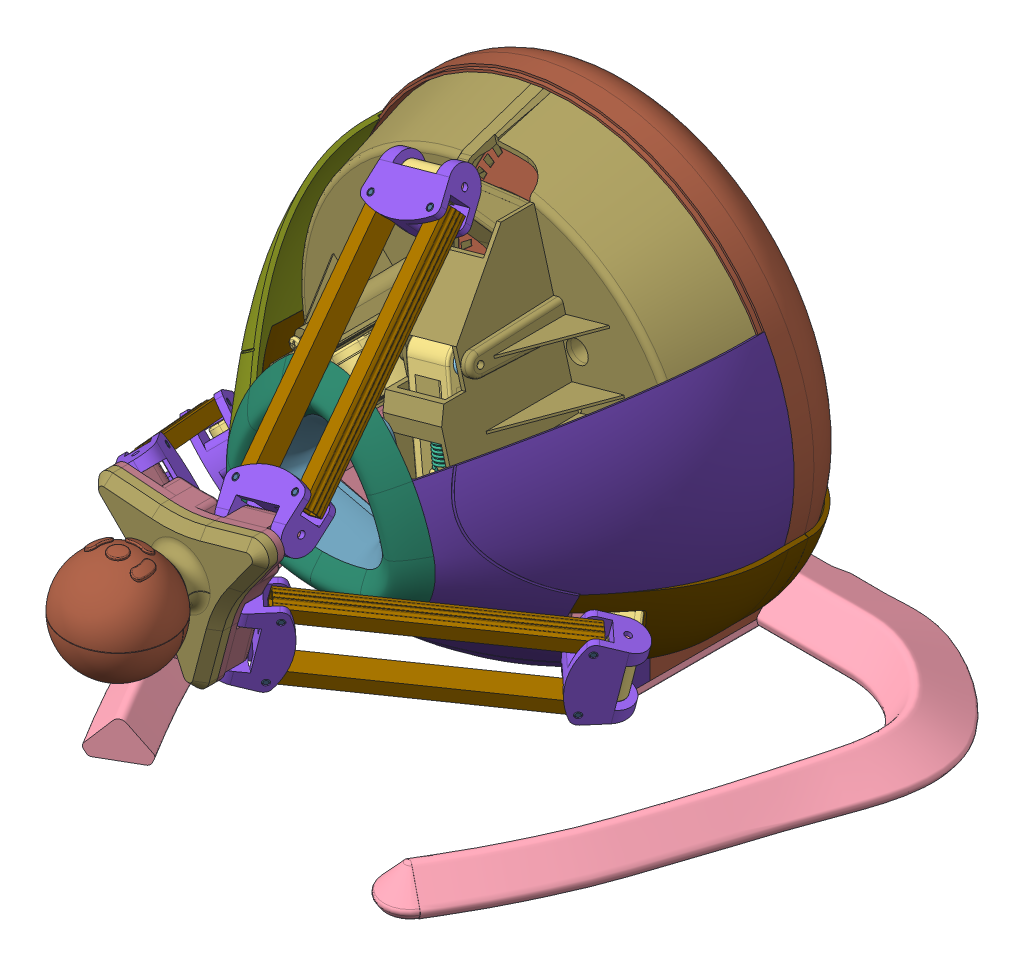
SolidWorks assembly ROBOT_SET_corr, configuration Défaut. Lengths in mm.
Overall size (305.26 266.62 319.84).
141 component instances, 33 part files, 47 mates.
Components (placement in the parent):
- bati-1: bati [Défaut] at (0 -115.25 -99.3181) size (305.26 272.51 243.47)
  - MOTEUR-1: MOTEUR [Défaut] at (0.3122 36.9309 38.5) x (-0.700162 -0.713984 0) z (0 0 -1) size (38 68 38)
  - FIXATION MOTEUR-1: FIXATION MOTEUR [Défaut] at (-16.4664 53.3847 38.5) x (-0.700162 -0.713984 0) z (0.713984 -0.700162 0) size (53.2 19.6 6)
  - FIXATION MOTEUR-2: FIXATION MOTEUR [Défaut] at (-38.9569 75.4398 38.5) x (-0.700162 -0.713984 0) z (0.713984 -0.700162 0) size (53.2 19.6 6)
  - Vis à tôle tête cylindrique cruciforme H 2,9x13 - C-1: Vis à tôle tête cylindrique cruciforme H 2,9x13 - C [Réaliste] at (-32.9202 36.6061 36.1) x (0 0 1) z (0.023398 -0.999726 0) size (14.76 5.6 5.6)
  - Vis à tôle tête cylindrique cruciforme H 2,9x13 - C-2: Vis à tôle tête cylindrique cruciforme H 2,9x13 - C [Réaliste] at (-55.4107 58.6612 36.1) x (0 0 1) z (0.704809 -0.709397 0) size (14.76 5.6 5.6)
  - Vis à tôle tête cylindrique cruciforme H 2,9x13 - C-3: Vis à tôle tête cylindrique cruciforme H 2,9x13 - C [Réaliste] at (-0.0126 70.1633 36.1) x (0 0 1) z (0.824881 -0.565307 0) size (14.76 5.6 5.6)
  - Vis à tôle tête cylindrique cruciforme H 2,9x13 - C-4: Vis à tôle tête cylindrique cruciforme H 2,9x13 - C [Réaliste] at (-22.5031 92.2184 36.1) x (0 0 1) z (0.309324 0.950957 0) size (14.76 5.6 5.6)
  - socle-1: socle [Défaut] at (0 -1.5 37.7) x (1 0 0) z (0 1 0) size (305.26 243.47 58.01)
  - vis CHC M4-30-1: vis CHC M4-30 [Défaut] at (9.875 31.2 14.05) x (-0.866025 0 0.5) z (0 -1 0) size (7 7 34)
  - vis CHC M4-30-2: vis CHC M4-30 [Défaut] at (-9.875 31.2 14.05) x (-0.866025 0 0.5) z (0 -1 0) size (7 7 34)
  - Rondelle M4-1: Rondelle M4 [Défaut] at (9.875 2 14.05) x (0.991496 0 -0.130134) z (-0.130134 0 -0.991496) size (9 0.8 9)
  - Rondelle M4-2: Rondelle M4 [Défaut] at (-9.875 1.2 14.05) x (0.991496 0 -0.130134) z (0.130134 0 0.991496) size (9 0.8 9)
  - CARTE HEXAGONALE-1: CARTE HEXAGONALE [Défaut] at (0 115.25 16.9) x (-0.956305 -0.292372 0) z (0 0 -1) size (138.56 120 30)
  - Vis à tôle tête cylindrique cruciforme H 2,9x13 - C-5: Vis à tôle tête cylindrique cruciforme H 2,9x13 - C [Réaliste] at (0 115.25 -1.8) x (0 0 1) z (1 0 0) size (14.76 5.6 5.6)
  - petite carte-1: petite carte [Défaut] at (-5.4923 106.1588 52.9) x (-0.224951 -0.97437 0) z (0 0 -1) size (34.7 16 10.5)
  - Vis à tôle tête cylindrique cruciforme H 2,9x8 - C-1: Vis à tôle tête cylindrique cruciforme H 2,9x8 - C [Réaliste] at (-6.6871 74.3113 49.1) x (0 0 1) z (-1 0 0) size (9.76 5.6 5.6)
  - Vis à tôle tête cylindrique cruciforme H 2,9x13 - C-7: Vis à tôle tête cylindrique cruciforme H 2,9x13 - C [Réaliste] at (13.5332 64.175 13.6) x (0 0 1) z (-1 0 0) size (14.76 5.6 5.6)
  - Vis à tôle tête cylindrique cruciforme H 2,9x8 - C-2: Vis à tôle tête cylindrique cruciforme H 2,9x8 - C [Réaliste] at (38.7975 129.9282 49.1) x (0 0 1) z (0.5 -0.866025 0) size (9.76 5.6 5.6)
  - Vis à tôle tête cylindrique cruciforme H 2,9x8 - C-3: Vis à tôle tête cylindrique cruciforme H 2,9x8 - C [Réaliste] at (-32.1104 141.5105 49.1) x (0 0 1) z (0.5 0.866025 0) size (9.76 5.6 5.6)
  - petite carte-2: petite carte [Défaut] at (10.6194 115.0391 52.9) x (0.956305 0.292372 0) z (0 0 -1) size (34.7 16 10.5)
  - petite carte-3: petite carte [Défaut] at (-5.1271 124.5521 52.9) x (-0.731354 0.681998 0) z (0 0 -1) size (34.7 16 10.5)
  - Vis à tôle tête cylindrique cruciforme H 2,9x13 - C-8: Vis à tôle tête cylindrique cruciforme H 2,9x13 - C [Réaliste] at (31.1975 107.2775 36.1) x (0 0 1) z (-0.978215 -0.207596 0) size (14.76 5.6 5.6)
  - Vis à tôle tête cylindrique cruciforme H 2,9x13 - C-9: Vis à tôle tête cylindrique cruciforme H 2,9x13 - C [Réaliste] at (-8.6944 146.2541 36.1) x (0 0 1) z (0.668891 -0.74336 0) size (14.76 5.6 5.6)
  - Vis à tôle tête cylindrique cruciforme H 2,9x13 - C-10: Vis à tôle tête cylindrique cruciforme H 2,9x13 - C [Réaliste] at (39.0525 137.7824 36.1) x (0 0 1) z (0.07713 0.997021 0) size (14.76 5.6 5.6)
  - Vis à tôle tête cylindrique cruciforme H 2,9x13 - C-11: Vis à tôle tête cylindrique cruciforme H 2,9x13 - C [Réaliste] at (-39.0399 137.8043 36.1) x (0 0 1) z (-0.90201 -0.431714 0) size (14.76 5.6 5.6)
  - Vis à tôle tête cylindrique cruciforme H 2,9x13 - C-12: Vis à tôle tête cylindrique cruciforme H 2,9x13 - C [Réaliste] at (76.7127 95.5573 36.1) x (0 0 1) z (0.261951 0.965081 0) size (14.76 5.6 5.6)
  - Vis à tôle tête cylindrique cruciforme H 2,9x13 - C-13: Vis à tôle tête cylindrique cruciforme H 2,9x13 - C [Réaliste] at (-21.302 191.5315 36.1) x (0 0 1) z (-0.96676 -0.255684 0) size (14.76 5.6 5.6)
  - Vis à tôle tête cylindrique cruciforme H 2,9x13 - C-14: Vis à tôle tête cylindrique cruciforme H 2,9x13 - C [Réaliste] at (84.5678 126.0622 36.1) x (0 0 1) z (0.854089 0.520126 0) size (14.76 5.6 5.6)
  - Vis à tôle tête cylindrique cruciforme H 2,9x13 - C-15: Vis à tôle tête cylindrique cruciforme H 2,9x13 - C [Réaliste] at (-51.6475 183.0817 36.1) x (0 0 1) z (-0.877487 0.4796 0) size (14.76 5.6 5.6)
  - MOTEUR-2: MOTEUR [Défaut] at (67.6702 154.6799 38.5) x (0.968409 -0.249366 0) z (0 0 -1) size (38 68 38)
  - MOTEUR-3: MOTEUR [Défaut] at (-67.9825 154.1392 38.5) x (-0.268247 0.96335 0) z (0 0 -1) size (38 68 38)
  - FIXATION MOTEUR-3: FIXATION MOTEUR [Défaut] at (53.9551 101.4174 38.5) x (0.968409 -0.249366 0) z (0.249366 0.968409 0) size (53.2 19.6 6)
  - FIXATION MOTEUR-4: FIXATION MOTEUR [Défaut] at (-14.9982 168.8928 38.5) x (-0.268247 0.96335 0) z (-0.96335 -0.268247 0) size (53.2 19.6 6)
  - Vis à tôle tête cylindrique cruciforme H 2,9x13 - C-16: Vis à tôle tête cylindrique cruciforme H 2,9x13 - C [Réaliste] at (37.4657 152.5076 13.6) x (0 0 1) z (0.5 -0.866025 0) size (14.76 5.6 5.6)
  - Vis à tôle tête cylindrique cruciforme H 2,9x13 - C-17: Vis à tôle tête cylindrique cruciforme H 2,9x13 - C [Réaliste] at (-50.9989 129.0674 13.6) x (0 0 1) z (0.5 0.866025 0) size (14.76 5.6 5.6)
  - plaque fixation-1: plaque fixation [Défaut] at origin size (50 130.5 32.4)
  - CARTER ARRIERE-1: CARTER ARRIERE [Défaut] x (-1 0 0) z (0 0 -1) size (201 215.75 63.51)
  - carter transparant-5: carter transparant [Défaut] at (53.7597 64.2778 0) x (0.999684 -0.02513 0) z (0 0 1) size (254.04 231.73 115.3)
    - carter transparant-1: carter transparant [Défaut] at (-154.833 107.2301 0) x (-0.5 -0.866025 0) z (0 0 1) size (168.6 94.54 100.3)
    - carter transparant2-1: carter transparant2 [Défaut] at (-55.0236 -65.6449 0) size (168.6 126.77 115.3)
    - carter transparant-2: carter transparant [Défaut] at (44.7858 107.2301 0) x (-0.5 0.866025 0) z (0 0 1) size (168.6 94.54 100.3)
  - Vis à tôle tête cylindrique cruciforme H 2,9x13 - C-18: Vis à tôle tête cylindrique cruciforme H 2,9x13 - C [Réaliste] at (78.1771 88.895 19.2) x (0 0 1) z (-0.823437 0.567408 0) size (14.76 5.6 5.6)
  - Vis à tôle tête cylindrique cruciforme H 2,9x13 - C-19: Vis à tôle tête cylindrique cruciforme H 2,9x13 - C [Réaliste] at (56.5905 55.2187 19.2) x (0 0 1) z (-1 0 0) size (14.76 5.6 5.6)
  - Vis à tôle tête cylindrique cruciforme H 2,9x13 - C-20: Vis à tôle tête cylindrique cruciforme H 2,9x13 - C [Réaliste] at (23.6934 194.2745 19.2) x (0 0 1) z (0.5 -0.866025 0) size (14.76 5.6 5.6)
  - Vis à tôle tête cylindrique cruciforme H 2,9x13 - C-21: Vis à tôle tête cylindrique cruciforme H 2,9x13 - C [Réaliste] at (-80.2839 96.2568 19.2) x (0 0 1) z (0.5 0.866025 0) size (14.76 5.6 5.6)
  - Vis à tôle tête cylindrique cruciforme H 2,9x13 - C-22: Vis à tôle tête cylindrique cruciforme H 2,9x13 - C [Réaliste] at (-16.2645 196.1309 19.2) x (0 0 1) z (-0.079672 -0.996821 0) size (14.76 5.6 5.6)
  - Vis à tôle tête cylindrique cruciforme H 2,9x13 - C-23: Vis à tôle tête cylindrique cruciforme H 2,9x13 - C [Réaliste] at (-61.9127 60.7241 19.2) x (0 0 1) z (0.903108 0.429413 0) size (14.76 5.6 5.6)
  - carter avant-1: carter avant [Défaut] at (17.1026 113.9098 24) size (270.48 238.53 119.64)
    - carter avant01-1: carter avant01 [Défaut] at (-17.1026 -113.9098 0) size (187.24 89.78 114.01) (hidden)
    - carter avant1-1: carter avant1 [Défaut] at (-17.1026 -113.9098 0) size (64.62 62.88 20.8)
    - CARTER NEZ-1: CARTER NEZ [Défaut] x (-1 0 0) z (0 1 0) size (94.64 9.63 92.67)
    - carter avant02-1: carter avant02 [Défaut] at (82.7068 58.9652 0) x (-0.5 0.866025 0) z (0 0 1) size (193.15 89.78 114.01)
    - carter avant03-1: carter avant03 [Défaut] at (-116.9121 58.9652 0) x (-0.5 -0.866025 0) z (0 0 1) size (191.25 89.78 114.01)
    - Vis à tôle tête cylindrique cruciforme H 2,9x13 - C-1: Vis à tôle tête cylindrique cruciforme H 2,9x13 - C [Réaliste] at (-32.0102 -41.9914 97) x (0 0 -1) z (1 0 0) size (14.76 5.6 5.6)
    - Vis à tôle tête cylindrique cruciforme H 2,9x13 - C-2: Vis à tôle tête cylindrique cruciforme H 2,9x13 - C [Réaliste] at (-47.1751 35.9163 97) x (0 0 -1) z (1 0 0) size (14.76 5.6 5.6)
    - Vis à tôle tête cylindrique cruciforme H 2,9x13 - C-3: Vis à tôle tête cylindrique cruciforme H 2,9x13 - C [Réaliste] at (27.8774 10.0956 97) x (0 0 -1) z (1 0 0) size (14.76 5.6 5.6)
  - FIXATION MOTEUR-5: FIXATION MOTEUR [Défaut] at (61.8101 131.9223 38.5) x (0.968409 -0.249366 0) z (0.249366 0.968409 0) size (53.2 19.6 6)
  - FIXATION MOTEUR-6: FIXATION MOTEUR [Défaut] at (-45.3437 160.443 38.5) x (-0.268247 0.96335 0) z (-0.96335 -0.268247 0) size (53.2 19.6 6)
  - PLAQUE NOM-1: PLAQUE NOM [Défaut] at (0 0 138) size (62.75 60.78 0.1) (hidden)
  - CACHE-1: CACHE [Défaut] at (0 0 24) size (77.2 40.92 103.91) (hidden)
  - CACHE-2: CACHE [Défaut] at (99.8094 172.875 24) x (-0.5 0.866025 0) z (0 0 1) size (77.2 40.92 103.91)
  - CACHE-3: CACHE [Défaut] at (-99.8094 172.875 24) x (-0.5 -0.866025 0) z (0 0 1) size (77.2 40.92 103.91)
- ROTOR-1: ROTOR [Défaut] at (-39.1783 46.9097 -60.8181) x (-0.96335 -0.268247 0) z (-0.263807 0.947405 -0.181189) size (89.6 91.37 91.37)
  - ROTOR-1: ROTOR [Défaut] at (30.9 0 0) x (0 0.28167 0.959511) z (0 -0.959511 0.28167) size (27 85 27)
  - ROUE CODEUSE-1: ROUE CODEUSE [Défaut] at (-36.4 0 0) x (0 0.892316 -0.451411) z (0 0.451411 0.892316) size (68 22.3 68)
- bras-6: bras [Défaut] at (-132.6949 -42.5944 -14.3424) x (-0.96335 -0.268247 0) z (0.042896 -0.154052 -0.987131) size (30 123.88 64.5)
  - bras-1: bras [Défaut] at (-166.5919 39.8256 -20.981) x (0 0 1) z (-1 0 0) size (64.5 123.88 20.1)
  - AXE BRAS-1: AXE BRAS [Défaut] at (-166.5919 39.8256 -20.981) x (0 0 -1) z (1 0 0) size (3 3 30)
  - palier bras-1: palier bras [Défaut] at origin size (5 10 10)
  - palier bras-2: palier bras [Défaut] at (-333.1838 5.2271 7.8152) x (-1 0 0) z (0 -0.924225 -0.381849) size (5 10 10)
  - Ressort cable-1: Ressort cable [Défaut] at (-166.5919 17.1829 -24.981) x (1 0 0) z (0 -1 0) size (9.03 7.82 23.53)
  - FIXATION CABLE-1: FIXATION CABLE [Défaut] at (-172.5919 90.5863 3.4188) x (1 0 0) z (0 0.85 0.526783) size (4 4 0.2)
- joint-10: joint [Défaut] at (-150.2793 16.6946 177.099) x (-0.96335 -0.268247 0) z (0.215805 -0.775014 0.593955) size (37.18 21.16 28.81)
  - joint-1: joint [Défaut] at (-167.6277 128.0999 -150.9355) x (1 0 0) z (0 -0.97714 -0.212597) size (37.18 26 16)
  - AXE BRAS-1: AXE BRAS [Défaut] at (-167.6277 126.3991 -143.1184) x (0 0 1) z (-1 0 0) size (3 3 30)
- BIELLE PARALLELOGRAMME-10: BIELLE PARALLELOGRAMME [Défaut] at (181.3565 63.4839 78.4276) x (0.967507 0.252134 0.018946) z (0.152652 -0.642213 0.751172) size (7.16 16 109)
  - BIELLE PARALLELOGRAMME-1: BIELLE PARALLELOGRAMME [Défaut] at (-178.1288 5 -54.5) x (0 -1 0) z (0 0 -1) size (10 7.16 109)
  - AXE BIELLE-1: AXE BIELLE [Défaut] at (-181.1288 5 -105.75) x (0.623444 0 0.781868) z (0 1 0) size (3 3 16)
  - AXE BIELLE-2: AXE BIELLE [Défaut] at (-181.1288 5 -3.25) x (0.623444 0 0.781868) z (0 1 0) size (3 3 16)
- BIELLE PARALLELOGRAMME-11: BIELLE PARALLELOGRAMME [Défaut] at (-144.1719 -13.104 78.1625) x (-0.967507 -0.252134 -0.018946) z (0.152652 -0.642213 0.751172) size (7.16 16 109)
  - BIELLE PARALLELOGRAMME-1: BIELLE PARALLELOGRAMME [Défaut] at (-178.1288 5 -54.5) x (0 -1 0) z (0 0 -1) size (10 7.16 109)
  - AXE BIELLE-1: AXE BIELLE [Défaut] at (-181.1288 5 -105.75) x (0.623444 0 0.781868) z (0 1 0) size (3 3 16)
  - AXE BIELLE-2: AXE BIELLE [Défaut] at (-181.1288 5 -3.25) x (0.623444 0 0.781868) z (0 1 0) size (3 3 16)
- joint-11: joint [Défaut] at (-152.1436 13.7551 -102.3866) x (-0.96335 -0.268247 0) z (-0.215805 0.775014 -0.593955) size (37.18 21.16 28.81)
  - joint-1: joint [Défaut] at (-167.6277 128.0999 -150.9355) x (1 0 0) z (0 -0.97714 -0.212597) size (37.18 26 16)
  - AXE BRAS-1: AXE BRAS [Défaut] at (-167.6277 126.3991 -143.1184) x (0 0 1) z (-1 0 0) size (3 3 30)
- ROTOR-2: ROTOR [Défaut] at (59.9648 9.506 -60.8181) x (0.249366 0.968409 0) z (0.867368 -0.223348 0.444734) size (89.6 91.37 91.37)
  - ROTOR-1: ROTOR [Défaut] at (30.9 0 0) x (0 0.28167 0.959511) z (0 -0.959511 0.28167) size (27 85 27)
  - ROUE CODEUSE-1: ROUE CODEUSE [Défaut] at (-36.4 0 0) x (0 0.892316 -0.451411) z (0 0.451411 0.892316) size (68 22.3 68)
- bras-5: bras [Défaut] at (29.4555 136.2153 -14.3296) x (0.249366 0.968409 0) z (-0.155146 0.03995 -0.987083) size (30 123.88 64.5)
  - bras-1: bras [Défaut] at (-166.5919 39.8256 -20.981) x (0 0 1) z (-1 0 0) size (64.5 123.88 20.1)
  - AXE BRAS-1: AXE BRAS [Défaut] at (-166.5919 39.8256 -20.981) x (0 0 -1) z (1 0 0) size (3 3 30)
  - palier bras-1: palier bras [Défaut] at origin size (5 10 10)
  - palier bras-2: palier bras [Défaut] at (-333.1838 5.2271 7.8152) x (-1 0 0) z (0 -0.924225 -0.381849) size (5 10 10)
  - Ressort cable-1: Ressort cable [Défaut] at (-166.5919 17.1829 -24.981) x (1 0 0) z (0 -1 0) size (9.03 7.82 23.53)
  - FIXATION CABLE-1: FIXATION CABLE [Défaut] at (-172.5919 90.5863 3.4188) x (1 0 0) z (0 0.85 0.526783) size (4 4 0.2)
- joint-12: joint [Défaut] at (89.6148 121.7939 177.0857) x (0.249366 0.968409 0) z (-0.77902 0.200598 0.594044) size (37.18 21.16 28.81)
  - joint-1: joint [Défaut] at (-167.6277 128.0999 -150.9355) x (1 0 0) z (0 -0.97714 -0.212597) size (37.18 26 16)
  - AXE BRAS-1: AXE BRAS [Défaut] at (-167.6277 126.3991 -143.1184) x (0 0 1) z (-1 0 0) size (3 3 30)
- BIELLE PARALLELOGRAMME-9: BIELLE PARALLELOGRAMME [Défaut] at (41.0818 -211.4151 2.4668) x (-0.262308 -0.964863 0.015282) z (0.633706 -0.18418 -0.751329) size (7.16 16 109)
  - BIELLE PARALLELOGRAMME-1: BIELLE PARALLELOGRAMME [Défaut] at (-178.1288 5 -54.5) x (0 -1 0) z (0 0 -1) size (10 7.16 109)
  - AXE BIELLE-1: AXE BIELLE [Défaut] at (-181.1288 5 -105.75) x (0.623444 0 0.781868) z (0 1 0) size (3 3 16)
  - AXE BIELLE-2: AXE BIELLE [Défaut] at (-181.1288 5 -3.25) x (0.623444 0 0.781868) z (0 1 0) size (3 3 16)
- BIELLE PARALLELOGRAMME-12: BIELLE PARALLELOGRAMME [Défaut] at (60.0485 131.074 78.8254) x (0.262308 0.964863 -0.015282) z (-0.633706 0.18418 0.751329) size (7.16 16 109)
  - BIELLE PARALLELOGRAMME-1: BIELLE PARALLELOGRAMME [Défaut] at (-178.1288 5 -54.5) x (0 -1 0) z (0 0 -1) size (10 7.16 109)
  - AXE BIELLE-1: AXE BIELLE [Défaut] at (-181.1288 5 -105.75) x (0.623444 0 0.781868) z (0 1 0) size (3 3 16)
  - AXE BIELLE-2: AXE BIELLE [Défaut] at (-181.1288 5 -3.25) x (0.623444 0 0.781868) z (0 1 0) size (3 3 16)
- joint-9: joint [Défaut] at (87.8395 124.4035 -102.391) x (0.249366 0.968409 0) z (0.77902 -0.200598 -0.594044) size (37.18 21.16 28.81)
  - joint-1: joint [Défaut] at (-167.6277 128.0999 -150.9355) x (1 0 0) z (0 -0.97714 -0.212597) size (37.18 26 16)
  - AXE BRAS-1: AXE BRAS [Défaut] at (-167.6277 126.3991 -143.1184) x (0 0 1) z (-1 0 0) size (3 3 30)
- ROTOR-3: ROTOR [Défaut] at (-21.7499 -56.6842 -60.8181) x (0.713984 -0.700162 0) z (0.616556 0.628727 0.473879) size (89.6 91.37 91.37)
  - ROTOR-1: ROTOR [Défaut] at (30.9 0 0) x (0 0.28167 0.959511) z (0 -0.959511 0.28167) size (27 85 27)
  - ROUE CODEUSE-1: ROUE CODEUSE [Défaut] at (-36.4 0 0) x (0 0.892316 -0.451411) z (0 0.451411 0.892316) size (68 22.3 68)
- bras-2: bras [Défaut] at (103.2352 -93.62 -14.3424) x (0.713984 -0.700162 0) z (0.111965 0.114175 -0.987131) size (30 123.88 64.5)
  - bras-1: bras [Défaut] at (-166.5919 39.8256 -20.981) x (0 0 1) z (-1 0 0) size (64.5 123.88 20.1)
  - AXE BRAS-1: AXE BRAS [Défaut] at (-166.5919 39.8256 -20.981) x (0 0 -1) z (1 0 0) size (3 3 30)
  - palier bras-1: palier bras [Défaut] at origin size (5 10 10)
  - palier bras-2: palier bras [Défaut] at (-333.1838 5.2271 7.8152) x (-1 0 0) z (0 -0.924225 -0.381849) size (5 10 10)
  - Ressort cable-1: Ressort cable [Défaut] at (-166.5919 17.1829 -24.981) x (1 0 0) z (0 -1 0) size (9.03 7.82 23.53)
  - FIXATION CABLE-1: FIXATION CABLE [Défaut] at (-172.5919 90.5863 3.4188) x (1 0 0) z (0 0.85 0.526783) size (4 4 0.2)
- joint-4: joint [Défaut] at (60.6817 -138.493 177.099) x (0.713984 -0.700162 0) z (0.563279 0.574399 0.593955) size (37.18 21.16 28.81)
  - joint-1: joint [Défaut] at (-167.6277 128.0999 -150.9355) x (1 0 0) z (0 -0.97714 -0.212597) size (37.18 26 16)
  - AXE BRAS-1: AXE BRAS [Défaut] at (-167.6277 126.3991 -143.1184) x (0 0 1) z (-1 0 0) size (3 3 30)
- BIELLE PARALLELOGRAMME-3: BIELLE PARALLELOGRAMME [Défaut] at (36.3921 -162.3501 -10.3136) x (0.702108 -0.711818 -0.018946) z (-0.479847 -0.453307 -0.751172) size (7.16 16 109)
  - BIELLE PARALLELOGRAMME-1: BIELLE PARALLELOGRAMME [Défaut] at (-178.1288 5 -54.5) x (0 -1 0) z (0 0 -1) size (10 7.16 109)
  - AXE BIELLE-1: AXE BIELLE [Défaut] at (-181.1288 5 -105.75) x (0.623444 0 0.781868) z (0 1 0) size (3 3 16)
  - AXE BIELLE-2: AXE BIELLE [Défaut] at (-181.1288 5 -3.25) x (0.623444 0 0.781868) z (0 1 0) size (3 3 16)
- BIELLE PARALLELOGRAMME-4: BIELLE PARALLELOGRAMME [Défaut] at (-203.2214 70.5419 3.1482) x (-0.702108 0.711818 0.018946) z (-0.479847 -0.453307 -0.751172) size (7.16 16 109)
  - BIELLE PARALLELOGRAMME-1: BIELLE PARALLELOGRAMME [Défaut] at (-178.1288 5 -54.5) x (0 -1 0) z (0 0 -1) size (10 7.16 109)
  - AXE BIELLE-1: AXE BIELLE [Défaut] at (-181.1288 5 -105.75) x (0.623444 0 0.781868) z (0 1 0) size (3 3 16)
  - AXE BIELLE-2: AXE BIELLE [Défaut] at (-181.1288 5 -3.25) x (0.623444 0 0.781868) z (0 1 0) size (3 3 16)
- joint-3: joint [Défaut] at (64.1594 -138.6378 -102.3866) x (0.713984 -0.700162 0) z (-0.563279 -0.574399 -0.593955) size (37.18 21.16 28.81)
  - joint-1: joint [Défaut] at (-167.6277 128.0999 -150.9355) x (1 0 0) z (0 -0.97714 -0.212597) size (37.18 26 16)
  - AXE BRAS-1: AXE BRAS [Défaut] at (-167.6277 126.3991 -143.1184) x (0 0 1) z (-1 0 0) size (3 3 30)
- poignee-1: poignee [Défaut] at (46.3334 -99.11 -94.3824) x (0.999684 -0.02513 0) z (0 0 1) size (91.69 95.36 94.16)
  - manette2-1: manette2 [Défaut] at (-49.9574 99.5142 190.1896) x (-0.954964 0.29672 0) z (0 0 1) size (46.3 47.3 60.42)
  - manette-1: manette [Default] at (-75.5797 129.3549 187.9639) x (-0.954964 0.29672 0) z (0 0 1) size (71.94 77.5 39.3)
    - manette1-1: manette1 [Défaut] at (-33.3227 20.8941 2.2257) size (71.94 77.5 39.3)
  - EFFECTEUR-1: EFFECTEUR [Défaut] at origin size (85.21 85.35 36.25)
    - BASE-1: BASE [Défaut] at (-48.8094 97.9143 187.1896) x (0.990623 -0.136626 0) z (0 0 1) size (75.58 75.74 36.25)
Mates (geometry in assembly coordinates):
- Coaxiale34: concentric anti-aligned: cylinder of joint-3/joint-1 through (-38.4577 16.1274 70.5751) axis (-0.526109 -0.536496 0.659834) radius 1.5; cylinder of BIELLE PARALLELOGRAMME-3/AXE BIELLE-1 through (-46.8755 7.5434 81.1324) axis (0.526109 0.536496 -0.659834) radius 1.5
- Coïncidente34: coincident anti-aligned: plane of joint-3/joint-1 through (-23.7775 11.102 90.3184) normal (0.526109 0.536496 -0.659834); plane of BIELLE PARALLELOGRAMME-3/AXE BIELLE-1 through (-42.6666 11.8354 75.8538) normal (-0.526109 -0.536496 0.659834)
- Coaxiale37: concentric aligned: cylinder of bras-2/bras-1 through (-94.1924 -42.7292 -9.5948) axis (0.713984 -0.700162 0) radius 1.5; cylinder of joint-4/AXE BRAS-1 through (-97.7623 -39.2284 -9.5948) axis (0.713984 -0.700162 0) radius 1.5
- Coïncidente37: coincident anti-aligned: plane of bras-2/bras-1 through (-45.5834 -7.4431 0) normal (-0.713984 0.700162 0); plane of joint-4/joint-1
- Coaxiale38: concentric aligned: cylinder of BIELLE PARALLELOGRAMME-3/AXE BIELLE-2 through (-96.0598 -38.9206 4.1373) axis (0.526109 0.536496 -0.659834) radius 1.5; cylinder of joint-4/joint-1 through (-96.0598 -38.9206 4.1373) axis (0.526109 0.536496 -0.659834) radius 1.5
- Coïncidente38: coincident anti-aligned: plane of BIELLE PARALLELOGRAMME-3/BIELLE PARALLELOGRAMME-1; plane of joint-4/joint-1 through (-90.7484 -53.4998 -15.6061) normal (-0.526109 -0.536496 0.659834)
- Coaxiale39: concentric aligned: cylinder of joint-3/joint-1 through (-18.4662 -3.4772 70.5751) axis (-0.526109 -0.536496 0.659834) radius 1.5; cylinder of BIELLE PARALLELOGRAMME-4/AXE BIELLE-1 through (-18.4662 -3.4772 70.5751) axis (-0.526109 -0.536496 0.659834) radius 1.5
- Coaxiale40: concentric anti-aligned: cylinder of BIELLE PARALLELOGRAMME-4/AXE BIELLE-2 through (-67.6505 -49.9412 -6.4201) axis (-0.526109 -0.536496 0.659834) radius 1.5; cylinder of joint-4/joint-1 through (-76.0682 -58.5251 4.1373) axis (0.526109 0.536496 -0.659834) radius 1.5
- Coïncidente39: coincident aligned: plane of BIELLE PARALLELOGRAMME-4/BIELLE PARALLELOGRAMME-1; plane of joint-4/joint-1 through (-90.7484 -53.4998 -15.6061) normal (-0.526109 -0.536496 0.659834)
- Coaxiale52: concentric aligned: cylinder of bras-5/bras-1 through (84.098 -60.2077 -9.6124) axis (0.249366 0.968409 0) radius 1.5; cylinder of joint-12/AXE BRAS-1 through (82.8511 -65.0498 -9.6124) axis (0.249366 0.968409 0) radius 1.5
- Coïncidente50: coincident anti-aligned: plane of bras-5/bras-1 through (29.2376 -35.7549 0) normal (-0.249366 -0.968409 0); plane of joint-12/joint-1
- Coaxiale53: concentric anti-aligned: cylinder of BIELLE PARALLELOGRAMME-12/AXE BIELLE-1 through (70.0908 -60.7313 -6.4363) axis (0.727744 -0.187395 0.659751) radius 1.5; cylinder of joint-12/joint-1 through (81.7347 -63.7297 4.1198) axis (-0.727744 0.187395 -0.659751) radius 1.5
- Coïncidente51: coincident anti-aligned: plane of BIELLE PARALLELOGRAMME-12/BIELLE PARALLELOGRAMME-1 through (82.398 -60.8715 -0.3472) normal (0.727744 -0.187395 0.659751); plane of joint-12/joint-1 through (101.4548 -54.3509 -19.5159) normal (-0.727744 0.187395 -0.659751)
- Coaxiale54: concentric anti-aligned: cylinder of BIELLE PARALLELOGRAMME-9/AXE BIELLE-2 through (77.0731 -33.6159 -6.4363) axis (0.727744 -0.187395 0.659751) radius 1.5; cylinder of joint-12/joint-1 through (88.717 -36.6142 4.1198) axis (-0.727744 0.187395 -0.659751) radius 1.5
- Coïncidente52: coincident anti-aligned: plane of BIELLE PARALLELOGRAMME-9/BIELLE PARALLELOGRAMME-1 through (18.7324 -19.4696 81.6394) normal (0.727744 -0.187395 0.659751); plane of joint-12/joint-1 through (101.4548 -54.3509 -19.5159) normal (-0.727744 0.187395 -0.659751)
- Coaxiale57: concentric aligned: cylinder of BIELLE PARALLELOGRAMME-12/AXE BIELLE-2 through (5.136 -41.8529 70.5749) axis (0.727744 -0.187395 0.659751) radius 1.5; cylinder of joint-9/joint-1 through (5.136 -41.8529 70.5749) axis (0.727744 -0.187395 0.659751) radius 1.5
- Coïncidente55: coincident anti-aligned: plane of BIELLE PARALLELOGRAMME-12/BIELLE PARALLELOGRAMME-1 through (75.1205 -58.9975 -6.9447) normal (-0.727744 0.187395 -0.659751); plane of joint-9/joint-1 through (-7.6019 -24.1162 94.2106) normal (0.727744 -0.187395 0.659751)
- Coaxiale59: concentric aligned: cylinder of BIELLE PARALLELOGRAMME-9/AXE BIELLE-1 through (12.1182 -14.7375 70.5749) axis (0.727744 -0.187395 0.659751) radius 1.5; cylinder of joint-9/joint-1 through (12.1182 -14.7375 70.5749) axis (0.727744 -0.187395 0.659751) radius 1.5
- Coaxiale60: concentric aligned: cylinder of bras-6/bras-1 through (10.0916 102.9375 -9.5948) axis (-0.96335 -0.268247 0) radius 1.5; cylinder of joint-10/AXE BRAS-1 through (14.9084 104.2788 -9.5948) axis (-0.96335 -0.268247 0) radius 1.5
- Coïncidente57: coincident anti-aligned: plane of bras-6/bras-1 through (16.3458 43.1979 0) normal (0.96335 0.268247 0); plane of joint-10/joint-1
- Coaxiale61: concentric anti-aligned: cylinder of BIELLE PARALLELOGRAMME-11/AXE BIELLE-1 through (17.5488 91.0685 -6.4201) axis (-0.201564 0.723872 0.659834) radius 1.5; cylinder of joint-10/joint-1 through (14.3237 102.6504 4.1373) axis (0.201564 -0.723872 -0.659834) radius 1.5
- Coïncidente58: coincident anti-aligned: plane of BIELLE PARALLELOGRAMME-11/BIELLE PARALLELOGRAMME-1 through (13.5454 94.5709 -6.9387) normal (0.201564 -0.723872 -0.659834); plane of joint-10/joint-1 through (-1.6436 107.8029 -26.0949) normal (-0.201564 0.723872 0.659834)
- Coaxiale62: concentric aligned: cylinder of BIELLE PARALLELOGRAMME-11/AXE BIELLE-2 through (33.1956 25.2416 70.5751) axis (-0.201564 0.723872 0.659834) radius 1.5; cylinder of joint-11/joint-1 through (33.1956 25.2416 70.5751) axis (-0.201564 0.723872 0.659834) radius 1.5
- Coïncidente59: coincident anti-aligned: plane of BIELLE PARALLELOGRAMME-11/BIELLE PARALLELOGRAMME-1 through (11.5298 101.8096 -0.3404) normal (-0.201564 0.723872 0.659834); plane of joint-11/joint-1 through (22.1892 12.5782 100.8072) normal (0.201564 -0.723872 -0.659834)
- Coaxiale63: concentric aligned: cylinder of BIELLE PARALLELOGRAMME-10/AXE BIELLE-1 through (-12.6501 95.1395 4.1373) axis (0.201564 -0.723872 -0.659834) radius 1.5; cylinder of joint-10/joint-1 through (-12.6501 95.1395 4.1373) axis (0.201564 -0.723872 -0.659834) radius 1.5
- Coïncidente60: coincident anti-aligned: plane of BIELLE PARALLELOGRAMME-10/BIELLE PARALLELOGRAMME-1 through (-9.639 95.8115 -0.2267) normal (-0.201564 0.723872 0.659834); plane of joint-10/joint-1 through (-3.6593 115.0417 -19.4965) normal (0.201564 -0.723872 -0.659834)
- Coaxiale64: concentric anti-aligned: cylinder of BIELLE PARALLELOGRAMME-10/AXE BIELLE-2 through (2.9968 29.3126 81.1324) axis (0.201564 -0.723872 -0.659834) radius 1.5; cylinder of joint-11/joint-1 through (6.2218 17.7307 70.5751) axis (-0.201564 0.723872 0.659834) radius 1.5
- Coaxiale65: concentric aligned: cylinder of bati-1/carter transparant-5/carter transparant2-1 through (7.8479 -118.8216 0) axis (0.249366 0.968409 0) radius 1.5; cylinder of bras-5/palier bras-2 through (33.1977 -20.376 0) axis (0.249366 0.968409 0) radius 3
- Coïncidente62: coincident anti-aligned: plane of bati-1/carter transparant-5/carter transparant2-1 through (66.6689 -57.2686 -39.4123) normal (0.249366 0.968409 0); plane of bras-5/palier bras-1 through (23.5022 -46.1532 0.4806) normal (-0.249366 -0.968409 0)
- Coïncidente63: coincident anti-aligned: plane of bati-1/carter transparant-5/carter transparant-2 through (16.2616 86.3712 -39.4123) normal (-0.96335 -0.268247 0); plane of bras-6/palier bras-1 through (28.2187 43.4299 0.4797) normal (0.96335 0.268247 0)
- Coaxiale66: concentric aligned: cylinder of bati-1/carter transparant-5/carter transparant-2 through (-50.2952 24.6415 0) axis (0.96335 0.268247 0) radius 1.5; cylinder of bras-6/palier bras-1 through (31.6444 47.4578 0) axis (0.96335 0.268247 0) radius 3
- Coaxiale67: concentric aligned: cylinder of bati-1/carter transparant-5/carter transparant-1 through (-106.8264 52.6143 0) axis (0.713984 -0.700162 0) radius 1.5; cylinder of bras-2/palier bras-2 through (-34.245 -18.5621 0) axis (0.713984 -0.700162 0) radius 3
- Coïncidente64: coincident anti-aligned: plane of bati-1/carter transparant-5/carter transparant-1 through (-24.324 -2.1888 -82.4181) normal (-0.713984 0.700162 0); plane of bras-2/palier bras-2 through (-36.2704 -14.371 -2.5538) normal (0.713984 -0.700162 0)
- Coaxiale73: concentric aligned: cylinder of bati-1/MOTEUR-1 through (0.3122 -78.3192 -60.8181) axis (0.713984 -0.700162 0) radius 19; cylinder of ROTOR-3/ROTOR-1 through (0.3122 -78.3192 -60.8181) axis (0.713984 -0.700162 0) radius 1.6
- Distance1: distance = 2.6 mm aligned: plane of bati-1/MOTEUR-1 through (-0.4239 -75.3564 -60.8181) normal (0.713984 -0.700162 0); plane of ROTOR-3/ROTOR-1 through (0.3122 -78.3192 -60.8181) normal (0.713984 -0.700162 0)
- Coaxiale74: concentric aligned: cylinder of bati-1/MOTEUR-3 through (-67.9825 38.8891 -60.8181) axis (-0.96335 -0.268247 0) radius 19; cylinder of ROTOR-1/ROTOR-1 through (-68.9458 38.6209 -60.8181) axis (-0.96335 -0.268247 0) radius 1.6
- Distance2: distance = 3.6 mm aligned: plane of ROTOR-1/ROTOR-1 through (-68.9458 38.6209 -60.8181) normal (-0.96335 -0.268247 0); plane of bati-1/MOTEUR-3 through (-65.0485 38.0452 -60.8181) normal (-0.96335 -0.268247 0)
- Coaxiale75: concentric aligned: cylinder of bati-1/MOTEUR-2 through (67.6702 39.4299 -60.8181) axis (0.249366 0.968409 0) radius 19; cylinder of ROTOR-2/ROTOR-1 through (67.6702 39.4299 -60.8181) axis (0.249366 0.968409 0) radius 13.5
- Distance3: distance = 2.6 mm aligned: plane of ROTOR-2/ROTOR-1 through (67.6702 39.4299 -60.8181) normal (0.249366 0.968409 0); plane of bati-1/MOTEUR-2 through (65.4724 37.311 -60.8181) normal (0.249366 0.968409 0)
- Coaxiale76: concentric aligned: cylinder of joint-3/AXE BRAS-1 through (-38.1832 17.8356 84.3071) axis (0.713984 -0.700162 0) radius 1.5; cylinder of poignee-1/EFFECTEUR-1/BASE-1 through (-48.2444 27.702 84.3071) axis (0.713984 -0.700162 0) radius 1.5
- Coïncidente73: coincident anti-aligned: plane of joint-3/joint-1 through (-35.9238 13.3554 97.6212) normal (0.713984 -0.700162 0); plane of poignee-1/EFFECTEUR-1/BASE-1 through (-38.2926 10.9399 84.3071) normal (-0.713984 0.700162 0)
- Coaxiale77: concentric aligned: cylinder of poignee-1/EFFECTEUR-1/BASE-1 through (38.2859 25.1935 84.3071) axis (-0.96335 -0.268247 0) radius 1.5; cylinder of joint-11/AXE BRAS-1 through (34.5377 24.1498 84.3071) axis (-0.96335 -0.268247 0) radius 1.5
- Coïncidente74: coincident anti-aligned: plane of poignee-1/EFFECTEUR-1/BASE-1 through (28.6205 27.6923 84.3071) normal (0.96335 0.268247 0); plane of joint-11/joint-1 through (29.528 24.4332 97.6212) normal (-0.96335 -0.268247 0)
- Coaxiale78: concentric aligned: cylinder of poignee-1/EFFECTEUR-1/BASE-1 through (1.9961 -48.3909 84.3071) axis (0.249366 0.968409 0) radius 1.5; cylinder of joint-9/AXE BRAS-1 through (3.5208 -42.4697 84.3071) axis (0.249366 0.968409 0) radius 1.5
- Coïncidente75: coincident anti-aligned: plane of poignee-1/EFFECTEUR-1/BASE-1 through (14.6594 -19.2642 84.3071) normal (0.249366 0.968409 0); plane of joint-9/joint-1 through (11.3845 -18.4209 97.621) normal (-0.249366 -0.968409 0)
- Angle4: planar angle = 1.727876 rad anti-aligned: plane of bras-6; plane of assembly through (0 0 0) normal (0 0 1)
- Coïncidente82: coincident aligned: line of ? through (0 0 156.2256) axis (0 0 1)
